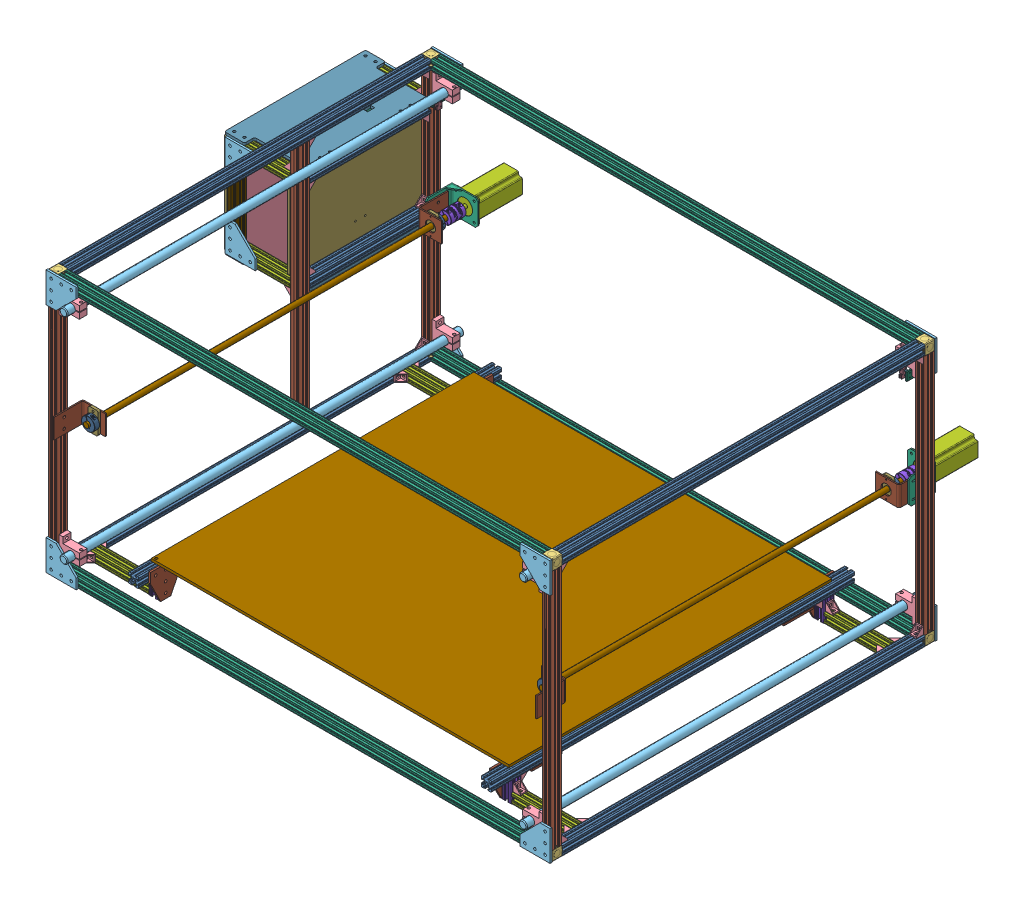
SolidWorks assembly Horizontal, configuration Default. Lengths in mm.
Overall size (1455.44 661.45 1123.18).
177 component instances, 33 part files, 21 mates.
Components (placement in the parent):
- Frame-1: Frame [Default] at origin size (1455.44 661.45 974.72)
  - Side Frame-1: Side Frame [Default] at origin size (76.73 661.45 974.72)
    - 3 ft-1: 3 ft [47065T412] at origin size (25.4 25.4 914.4)
    - 3 ft-2: 3 ft [47065T412] at (0 635 0) size (25.4 25.4 914.4)
    - 2 ft-3: 2 ft [47065T209] at (0 317.5 469.9) x (1 0 0) z (0 -1 0) size (25.4 25.4 609.6)
    - 2 ft-4: 2 ft [47065T209] at (0 317.5 -469.9) x (1 0 0) z (0 1 0) size (25.4 25.4 609.6)
    - Outside Corner-1: Outside Corner [47065T244] at (12.7 622.3 457.2) x (0 0 1) z (-1 0 0) size (28.42 28.42 28.42)
    - Outside Corner-2: Outside Corner [47065T244] at (12.7 622.3 -457.2) x (0 1 0) z (-1 0 0) size (28.42 28.42 28.42)
    - Outside Corner-3: Outside Corner [47065T244] at (12.7 12.7 457.2) x (0 -1 0) z (-1 0 0) size (28.42 28.42 28.42)
    - Outside Corner-4: Outside Corner [47065T244] at (12.7 12.7 -457.2) x (-1 0 0) z (0 -1 0) size (28.42 28.42 28.42)
    - Corner Brace-1: Corner Brace [47065T216] at (0 12.7 457.2) x (0 0 -1) z (1 0 0) size (19.81 19.81 18)
    - Corner Brace-2: Corner Brace [47065T216] at (0 12.7 -457.2) x (0 0 1) z (-1 0 0) size (19.81 19.81 18)
    - Corner Brace-3: Corner Brace [47065T216] at (0 622.3 -457.2) x (0 -1 0) z (-1 0 0) size (19.81 19.81 18)
    - Corner Brace-4: Corner Brace [47065T216] at (0 622.3 457.2) x (0 0 -1) z (-1 0 0) size (19.81 19.81 18)
    - Corner Surface-1: Corner Surface [47065T267] at (-12.7 647.7 484.9812) x (0 -1 0) z (0 0 1) size (76.2 76.2 4.76)
    - Corner Surface-3: Corner Surface [47065T267] at (-12.7 -12.7 -484.9812) size (76.2 76.2 4.76)
    - Corner Surface-4: Corner Surface [47065T267] at (-12.7 -12.7 484.9812) size (76.2 76.2 4.76)
    - Corner Surface-5: Corner Surface [47065T267] at (-12.7 647.7 -484.9812) x (0 -1 0) z (0 0 1) size (76.2 76.2 4.76)
  - 4 ft-1: 4 ft [47065T121] at (622.3 0 469.9) x (0 0 1) z (-1 0 0) size (25.4 25.4 1219.2)
  - 4 ft-2: 4 ft [47065T121] at (622.3 635 469.9) x (0 0 1) z (-1 0 0) size (25.4 25.4 1219.2)
  - 4 ft-3: 4 ft [47065T121] at (622.3 635 -469.9) x (0 0 -1) z (1 0 0) size (25.4 25.4 1219.2)
  - 4 ft-4: 4 ft [47065T121] at (622.3 0 -469.9) x (0 0 -1) z (1 0 0) size (25.4 25.4 1219.2)
  - Side Frame-2: Side Frame [Default] at (1244.6 0 0) x (-1 0 0) z (0 0 -1) size (76.73 661.45 974.72)
    - 3 ft-1: 3 ft [47065T412] at origin size (25.4 25.4 914.4)
    - 3 ft-2: 3 ft [47065T412] at (0 635 0) size (25.4 25.4 914.4)
    - 2 ft-3: 2 ft [47065T209] at (0 317.5 469.9) x (1 0 0) z (0 -1 0) size (25.4 25.4 609.6)
    - 2 ft-4: 2 ft [47065T209] at (0 317.5 -469.9) x (1 0 0) z (0 1 0) size (25.4 25.4 609.6)
    - Outside Corner-1: Outside Corner [47065T244] at (12.7 622.3 457.2) x (0 0 1) z (-1 0 0) size (28.42 28.42 28.42)
    - Outside Corner-2: Outside Corner [47065T244] at (12.7 622.3 -457.2) x (0 1 0) z (-1 0 0) size (28.42 28.42 28.42)
    - Outside Corner-3: Outside Corner [47065T244] at (12.7 12.7 457.2) x (0 -1 0) z (-1 0 0) size (28.42 28.42 28.42)
    - Outside Corner-4: Outside Corner [47065T244] at (12.7 12.7 -457.2) x (-1 0 0) z (0 -1 0) size (28.42 28.42 28.42)
    - Corner Brace-1: Corner Brace [47065T216] at (0 12.7 457.2) x (0 0 -1) z (1 0 0) size (19.81 19.81 18)
    - Corner Brace-2: Corner Brace [47065T216] at (0 12.7 -457.2) x (0 0 1) z (-1 0 0) size (19.81 19.81 18)
    - Corner Brace-3: Corner Brace [47065T216] at (0 622.3 -457.2) x (0 -1 0) z (-1 0 0) size (19.81 19.81 18)
    - Corner Brace-4: Corner Brace [47065T216] at (0 622.3 457.2) x (0 0 -1) z (-1 0 0) size (19.81 19.81 18)
    - Corner Surface-1: Corner Surface [47065T267] at (-12.7 647.7 484.9812) x (0 -1 0) z (0 0 1) size (76.2 76.2 4.76)
    - Corner Surface-3: Corner Surface [47065T267] at (-12.7 -12.7 -484.9812) size (76.2 76.2 4.76)
    - Corner Surface-4: Corner Surface [47065T267] at (-12.7 -12.7 484.9812) size (76.2 76.2 4.76)
    - Corner Surface-5: Corner Surface [47065T267] at (-12.7 647.7 -484.9812) x (0 -1 0) z (0 0 1) size (76.2 76.2 4.76)
  - 6 in-1: 6 in [47065T411] at (88.9 0 393.7) x (0 0 1) z (-1 0 0) size (25.4 25.4 152.4)
  - 2 in-3: 2 in [47065T411] at (177.8 12.7 393.7) x (1 0 0) z (0 -1 0) size (25.4 25.4 50.8)
  - 6 in-2: 6 in [47065T411] at (88.9 0 -393.7) x (0 0 -1) z (1 0 0) size (25.4 25.4 152.4)
  - 2 in-4: 2 in [47065T411] at (177.8 12.7 -393.7) x (1 0 0) z (0 1 0) size (25.4 25.4 50.8)
  - 3 ft-1: 3 ft [47065T412] at (177.8 50.8 0) size (25.4 25.4 914.4)
  - 3 ft-2: 3 ft [47065T412] at (1066.8 50.8 0) x (-1 0 0) z (0 0 -1) size (25.4 25.4 914.4)
  - 2 in-7: 2 in [47065T411] at (1066.8 12.7 393.7) x (-1 0 0) z (0 1 0) size (25.4 25.4 50.8)
  - 6 in-5: 6 in [47065T411] at (1155.7 0 393.7) x (0 0 1) z (-1 0 0) size (25.4 25.4 152.4)
  - 6 in-6: 6 in [47065T411] at (1155.7 0 -393.7) x (0 0 -1) z (1 0 0) size (25.4 25.4 152.4)
  - 2 in-8: 2 in [47065T411] at (1066.8 12.7 -393.7) x (-1 0 0) z (0 -1 0) size (25.4 25.4 50.8)
  - PVC Panel-1: PVC Panel [Default] at (622.3 66.675 0) size (901.7 6.35 812.8)
  - 34in-1: 34in [47065T412] at (622.3 50.8 -317.5) x (0 0 1) z (-1 0 0) size (25.4 25.4 863.6)
  - 34in-2: 34in [47065T412] at (622.3 50.8 317.5) x (0 0 1) z (-1 0 0) size (25.4 25.4 863.6)
  - 2 ft-1: 2 ft [47065T209] at (622.3 50.8 0) size (25.4 25.4 609.6)
  - Corner Brace-2: Corner Brace [47065T216] at (165.1 12.7 393.7) x (-1 0 0) z (0 0 -1) size (19.81 19.81 18)
  - Corner Brace-3: Corner Brace [47065T216] at (12.7 0 381) x (1 0 0) z (0 1 0) size (19.81 19.81 18)
  - Corner Brace-4: Corner Brace [47065T216] at (12.7 0 406.4) x (1 0 0) z (0 -1 0) size (19.81 19.81 18)
  - Corner Brace-5: Corner Brace [47065T216] at (177.8 38.1 381) x (0 -1 0) z (1 0 0) size (19.81 19.81 18)
  - Corner Brace-6: Corner Brace [47065T216] at (190.5 50.8 304.8) x (1 0 0) z (0 1 0) size (19.81 19.81 18)
  - Surface T-1: Surface T [47065T278] at (192.8812 63.5 355.6) x (0 0 1) z (1 0 0) size (76.2 76.2 4.76)
  - Surface T-2: Surface T [47065T278] at (165.1 35.7188 279.4) x (0 0 1) z (0 1 0) size (76.2 76.2 4.76)
  - Corner Brace-7: Corner Brace [47065T216] at (12.7 0 -406.4) x (1 0 0) z (0 1 0) size (19.81 19.81 18)
  - Corner Brace-8: Corner Brace [47065T216] at (12.7 0 -381) x (1 0 0) z (0 -1 0) size (19.81 19.81 18)
  - Corner Brace-9: Corner Brace [47065T216] at (165.1 12.7 -393.7) x (-1 0 0) z (0 0 -1) size (19.81 19.81 18)
  - Surface T-3: Surface T [47065T278] at (192.8812 63.5 -355.6) x (0 0 -1) z (-1 0 0) size (76.2 76.2 4.76)
  - Corner Brace-10: Corner Brace [47065T216] at (177.8 38.1 -381) x (0 -1 0) z (-1 0 0) size (19.81 19.81 18)
  - Surface T-4: Surface T [47065T278] at (165.1 35.7188 -279.4) x (0 0 -1) z (0 -1 0) size (76.2 76.2 4.76)
  - Corner Brace-11: Corner Brace [47065T216] at (190.5 50.8 -304.8) x (1 0 0) z (0 -1 0) size (19.81 19.81 18)
  - Corner Brace-12: Corner Brace [47065T216] at (609.6 50.8 304.8) x (-1 0 0) z (0 -1 0) size (19.81 19.81 18)
  - Surface T-5: Surface T [47065T278] at (660.4 35.7188 330.2) x (-1 0 0) z (0 -1 0) size (76.2 76.2 4.76)
  - Surface T-6: Surface T [47065T278] at (660.4 35.7188 -330.2) x (-1 0 0) z (0 1 0) size (76.2 76.2 4.76)
  - Corner Brace-13: Corner Brace [47065T216] at (609.6 50.8 -304.8) x (-1 0 0) z (0 1 0) size (19.81 19.81 18)
  - Corner Brace-14: Corner Brace [47065T216] at (1231.9 0 381) x (-1 0 0) z (0 -1 0) size (19.81 19.81 18)
  - Corner Brace-15: Corner Brace [47065T216] at (1231.9 0 406.4) x (-1 0 0) z (0 1 0) size (19.81 19.81 18)
  - Corner Brace-16: Corner Brace [47065T216] at (1231.9 0 -381) x (-1 0 0) z (0 1 0) size (19.81 19.81 18)
  - Corner Brace-17: Corner Brace [47065T216] at (1231.9 0 -406.4) x (-1 0 0) z (0 -1 0) size (19.81 19.81 18)
  - Surface T-7: Surface T [47065T278] at (1051.7188 63.5 -355.6) x (0 0 -1) z (-1 0 0) size (76.2 76.2 4.76)
  - Surface T-8: Surface T [47065T278] at (1051.7188 63.5 355.6) x (0 0 1) z (1 0 0) size (76.2 76.2 4.76)
  - Surface T-9: Surface T [47065T278] at (1079.5 35.7188 279.4) x (0 0 1) z (0 -1 0) size (76.2 76.2 4.76)
  - Surface T-10: Surface T [47065T278] at (1079.5 35.7188 -279.4) x (0 0 -1) z (0 1 0) size (76.2 76.2 4.76)
  - Corner Brace-18: Corner Brace [47065T216] at (1054.1 50.8 -304.8) x (-1 0 0) z (0 1 0) size (19.81 19.81 18)
  - Corner Brace-19: Corner Brace [47065T216] at (1054.1 50.8 304.8) x (-1 0 0) z (0 -1 0) size (19.81 19.81 18)
  - Corner Brace-20: Corner Brace [47065T216] at (1066.8 38.1 381) x (0 -1 0) z (1 0 0) size (19.81 19.81 18)
  - Corner Brace-21: Corner Brace [47065T216] at (1079.5 12.7 393.7) size (19.81 19.81 18)
  - Corner Brace-22: Corner Brace [47065T216] at (1079.5 12.7 -393.7) size (19.81 19.81 18)
  - Corner Brace-23: Corner Brace [47065T216] at (1066.8 38.1 -381) x (0 -1 0) z (-1 0 0) size (19.81 19.81 18)
  - Corner Brace-24: Corner Brace [47065T216] at (635 50.8 304.8) x (1 0 0) z (0 1 0) size (19.81 19.81 18)
  - Corner Brace-25: Corner Brace [47065T216] at (635 50.8 -304.8) x (1 0 0) z (0 -1 0) size (19.81 19.81 18)
  - Electronics Box-1: Electronics Box [Default] at (-12.7 426.5 -304.8) x (0 0 1) z (0 -1 0) size (365.12 210.31 613.21)
    - Box Bottom-1: Box Bottom [Bottom] at origin size (355.6 6.35 254)
    - Box Bottom-2: Box Bottom [Top] at (0 158.75 0) size (355.6 6.35 254)
    - Box Left-1: Box Left [Left] at (-152.4 82.55 0) x (0 0 -1) z (0 -1 0) size (254 6.35 152.4)
    - Box Left-2: Box Left [Right] at (146.05 82.55 0) x (0 0 -1) z (0 -1 0) size (254 6.35 152.4)
    - Box Front-3: Box Front [Default] at (0 69.85 127) size (355.6 190.5 6.35)
    - Box Front-4: Box Front [Back] at (0 69.85 -133.35) size (355.6 190.5 6.35)
    - Motor Drive-1: Motor Drive [Default] at (-106.05 71.23 -104.32) x (0 -1 0) z (-1 0 0) size (120 33 80)
    - Motor Drive-2: Motor Drive [Default] at (-106.05 71.23 -61.14) x (0 -1 0) z (-1 0 0) size (120 33 80)
    - Motor Drive-3: Motor Drive [Default] at (-106.05 71.23 25.22) x (0 -1 0) z (-1 0 0) size (120 33 80)
    - Motor Drive-4: Motor Drive [Default] at (-106.05 71.23 -17.96) x (0 -1 0) z (-1 0 0) size (120 33 80)
    - PSU-1: PSU [Default] at (-25 63.85 -12.7) x (0 0 -1) z (0 -1 0) size (215 50 115)
    - pi-1: pi [Default] at (80.934 6.35 15.1253) x (-1 0 0) z (0 0 -1) size (93.98 91.95 116.84)
    - Box Side Frame-1: Box Side Frame [Default] at (-165.1 146.05 0) x (-1 0 0) z (0 0 -1) size (30.16 160.56 290)
      - 8 in-1: 8 in [47065T411] at origin size (25.4 25.4 203.2)
      - 6 in-1: 6 in [47065T411] at (0 -69.85 114.3) x (1 0 0) z (0 -1 0) size (25.4 25.4 152.4)
      - 6 in-2: 6 in [47065T411] at (0 -69.85 -114.3) x (1 0 0) z (0 1 0) size (25.4 25.4 152.4)
      - Corner Surface-1: Corner Surface [47065T267] at (15.0812 12.7 127) x (0 -1 0) z (1 0 0) size (76.2 76.2 4.76)
      - Corner Surface-2: Corner Surface [47065T267] at (15.0812 12.7 -127) x (0 0 1) z (1 0 0) size (76.2 76.2 4.76)
      - Corner Brace-1: Corner Brace [47065T216] at (0 -146.05 127) x (0 0 1) z (-1 0 0) size (19.81 19.81 18)
      - Corner Brace-2: Corner Brace [47065T216] at (0 -146.05 -127) x (0 0 -1) z (1 0 0) size (19.81 19.81 18)
    - Box Side Frame-2: Box Side Frame [Default] at (165.1 146.05 0) size (30.16 160.56 290)
      - 8 in-1: 8 in [47065T411] at origin size (25.4 25.4 203.2)
      - 6 in-1: 6 in [47065T411] at (0 -69.85 114.3) x (1 0 0) z (0 -1 0) size (25.4 25.4 152.4)
      - 6 in-2: 6 in [47065T411] at (0 -69.85 -114.3) x (1 0 0) z (0 1 0) size (25.4 25.4 152.4)
      - Corner Surface-1: Corner Surface [47065T267] at (15.0812 12.7 127) x (0 -1 0) z (1 0 0) size (76.2 76.2 4.76)
      - Corner Surface-2: Corner Surface [47065T267] at (15.0812 12.7 -127) x (0 0 1) z (1 0 0) size (76.2 76.2 4.76)
      - Corner Brace-1: Corner Brace [47065T216] at (0 -146.05 127) x (0 0 1) z (-1 0 0) size (19.81 19.81 18)
      - Corner Brace-2: Corner Brace [47065T216] at (0 -146.05 -127) x (0 0 -1) z (1 0 0) size (19.81 19.81 18)
    - 2 ft-2: 2 ft [47065T209] at (165.1 -12.7 109) size (25.4 25.4 609.6)
    - 1 ft-3: 1 ft [47065T411] at (0 -12.7 114.3) x (0 0 1) z (-1 0 0) size (25.4 25.4 304.8)
    - Corner Brace-9: Corner Brace [47065T216] at (-152.4 -12.7 101.6) x (0 0 -1) z (0 -1 0) size (19.81 19.81 18)
    - Corner Brace-10: Corner Brace [47065T216] at (152.4 -12.7 101.6) x (0 0 -1) z (0 1 0) size (19.81 19.81 18)
    - 1 ft-4: 1 ft [47065T411] at (0 -12.7 -114.3) x (0 0 -1) z (1 0 0) size (25.4 25.4 304.8)
    - Corner Brace-13: Corner Brace [47065T216] at (-152.4 -12.7 -101.6) x (0 0 1) z (0 1 0) size (19.81 19.81 18)
    - Corner Brace-14: Corner Brace [47065T216] at (152.4 -12.7 -101.6) x (-1 0 0) z (0 1 0) size (19.81 19.81 18)
    - Corner Brace-15: Corner Brace [47065T216] at (152.4 -12.7 -195.8) x (0 0 1) z (0 -1 0) size (19.81 19.81 18)
    - Corner Brace-16: Corner Brace [47065T216] at (152.4 -12.7 413.8) x (-1 0 0) z (0 -1 0) size (19.81 19.81 18)
    - Switch-1: Switch [7343K291] at (25.4 158.75 -76.2) x (0 0 -1) z (1 0 0) size (31.31 51.82 16)
    - Switch-2: Switch [7343K291] at (63.5 158.75 -76.2) x (0 0 -1) z (1 0 0) size (31.31 51.82 16)
    - Switch-3: Switch [7343K291] at (101.6 158.75 -76.2) x (0 0 -1) z (1 0 0) size (31.31 51.82 16)
    - Switch Holder-1: Switch Holder [Default] at (63.5 156.083 -76.2) size (152.4 5.33 63.5)
- Horizontal Rail-1: Horizontal Rail [Default] at (12.7 79.125 469.9) x (0 -1 0) z (0 0 1) size (60 51 1000)
  - Shaft Clamp 20mm-1: Shaft Clamp 20mm [Default] at (0 0 -939.8) size (60 51 20)
  - Shaft 1000mm-1: Shaft 1000mm [6459K62] at (30 31 -469.9) x (-0.976033 -0.217622 0) z (0 0 1) size (20 20 1000)
  - Shaft Clamp 20mm-11: Shaft Clamp 20mm [Default] at origin size (60 51 20)
- Horizontal Motor-1: Horizontal Motor [Default] at (48.2 319.125 -510.1768) x (0 -1 0) z (0 0 1) size (65 68 1118.48)
  - Motor Mount-1: Motor Mount [Default] at origin size (65 68 68)
  - Nema 23 Stepper Motor-1: Nema 23 Stepper Motor [Default] at (28.5 -28.5 0) x (0 0 -1) z (1 0 0) size (137 57 57)
  - Shaft Coupler-1: Shaft Coupler [2464K34] at (0 0 33.602) x (-0.85098 -0.525198 0) z (0 0 -1) size (30 30.01 38)
  - Lead Screw 3ft-2: Lead Screw 3ft [Default] at (0 0 500.404) x (0 0 1) z (0.598663 0.801001 0) size (914.4 12.7 12.7)
  - Collar-1: Collar [6698K13] at (0 0 74.1796) x (0.295803 -0.955249 0) z (0 0 1) size (33.3 33.27 13.41)
  - Collar-2: Collar [6698K13] at (0 0 946.174) x (0.943106 0.332491 0) z (0 0 1) size (33.3 33.27 13.41)
  - L Bracket-1: L Bracket [Without Motor] at (25 -35.5 930.4768) x (0 0 1) z (-1 0 0) size (75 59.99 50)
  - L Bracket-2: L Bracket [With Motor] at (-25 -32.5 89.8768) x (0 0 -1) z (1 0 0) size (75 59.99 50)
  - Acrylic Bearing Mount-1: Acrylic Bearing Mount [Default] at (0 0 936.649) size (55.88 25.4 6.35)
  - Acrylic Bearing Mount-2: Acrylic Bearing Mount [Default] at (0 0 83.7046) size (55.88 25.4 6.35)
- Horizontal Rail-3: Horizontal Rail [Default] at (12.7 619.125 469.9) x (0 -1 0) z (0 0 1) size (60 51 1000)
  - Shaft Clamp 20mm-1: Shaft Clamp 20mm [Default] at (0 0 -939.8) size (60 51 20)
  - Shaft 1000mm-1: Shaft 1000mm [6459K62] at (30 31 -469.9) x (-0.976033 -0.217622 0) z (0 0 1) size (20 20 1000)
  - Shaft Clamp 20mm-11: Shaft Clamp 20mm [Default] at origin size (60 51 20)
- Limit Swtich Assembly 2-1: Limit Swtich Assembly 2 [Default] at (1221.9 571.6895 -443.7567) x (0 0 -1) z (0 1 0) size (15.52 14.29 21.84)
  - Limit Switch-2: Limit Switch [Default] at (13.2909 14.2875 -7.4832) x (0 0 1) z (0 -1 0) size (21.84 15.52 6.35)
  - Standoff-1: Standoff [90268A203] at (10.9033 11.1125 -2.7207) x (0.90245 0 -0.430795) z (0 1 0) size (4.76 5.5 7.94)
  - Standoff-2: Standoff [90268A203] at (10.9033 11.1125 -12.2457) x (0.948451 0 0.316923) z (0 1 0) size (4.76 5.5 7.94)
- Horizontal Rail-4: Horizontal Rail [Default] at (1231.9 79.125 -469.9) x (0 -1 0) z (0 0 -1) size (60 51 1000)
  - Shaft Clamp 20mm-1: Shaft Clamp 20mm [Default] at (0 0 -939.8) size (60 51 20)
  - Shaft 1000mm-1: Shaft 1000mm [6459K62] at (30 31 -469.9) x (-0.976033 -0.217622 0) z (0 0 1) size (20 20 1000)
  - Shaft Clamp 20mm-11: Shaft Clamp 20mm [Default] at origin size (60 51 20)
- Horizontal Motor-2: Horizontal Motor [Default] at (1196.4 319.125 -510.1768) x (0 1 0) z (0 0 1) size (65 68 1118.48)
  - Motor Mount-1: Motor Mount [Default] at origin size (65 68 68)
  - Nema 23 Stepper Motor-1: Nema 23 Stepper Motor [Default] at (28.5 -28.5 0) x (0 0 -1) z (1 0 0) size (137 57 57)
  - Shaft Coupler-1: Shaft Coupler [2464K34] at (0 0 33.602) x (-0.85098 -0.525198 0) z (0 0 -1) size (30 30.01 38)
  - Lead Screw 3ft-2: Lead Screw 3ft [Default] at (0 0 500.404) x (0 0 1) z (0.598663 0.801001 0) size (914.4 12.7 12.7)
  - Collar-1: Collar [6698K13] at (0 0 74.1796) x (0.295803 -0.955249 0) z (0 0 1) size (33.3 33.27 13.41)
  - Collar-2: Collar [6698K13] at (0 0 946.174) x (0.943106 0.332491 0) z (0 0 1) size (33.3 33.27 13.41)
  - L Bracket-1: L Bracket [Without Motor] at (25 -35.5 930.4768) x (0 0 1) z (-1 0 0) size (75 59.99 50)
  - L Bracket-2: L Bracket [With Motor] at (-25 -32.5 89.8768) x (0 0 -1) z (1 0 0) size (75 59.99 50)
  - Acrylic Bearing Mount-1: Acrylic Bearing Mount [Default] at (0 0 936.649) size (55.88 25.4 6.35)
  - Acrylic Bearing Mount-2: Acrylic Bearing Mount [Default] at (0 0 83.7046) size (55.88 25.4 6.35)
- Horizontal Rail-5: Horizontal Rail [Default] at (1231.9 619.125 -469.9) x (0 -1 0) z (0 0 -1) size (60 51 1000)
  - Shaft Clamp 20mm-1: Shaft Clamp 20mm [Default] at (0 0 -939.8) size (60 51 20)
  - Shaft 1000mm-1: Shaft 1000mm [6459K62] at (30 31 -469.9) x (-0.976033 -0.217622 0) z (0 0 1) size (20 20 1000)
  - Shaft Clamp 20mm-11: Shaft Clamp 20mm [Default] at origin size (60 51 20)
- Limit Swtich Assembly 1-2: Limit Swtich Assembly 1 [Default] at (21.8635 571.2553 -445.7389) x (0 0 -1) z (0 1 0) size (15.52 14.29 21.84)
  - Limit Switch-2: Limit Switch [Default] at (11.3087 -15.124 -7.049) x (0 0 1) z (0 -1 0) size (21.84 15.52 6.35)
  - Standoff-1: Standoff [90268A203] at (8.9211 -4.0115 -2.2865) x (0.645868 0 0.763449) z (0 1 0) size (4.76 5.5 7.94)
  - Standoff-2: Standoff [90268A203] at (8.9211 -4.0115 -11.8115) x (0.926416 0 0.3765) z (0 1 0) size (4.76 5.5 7.94)
- Al sheet 4-1-1: Al sheet 4-1 [Default] at (1221.9 574.125 -446.88) x (0 0 -1) z (0 1 0) size (33.02 3.17 20.32)
- Al sheet 4-1-2: Al sheet 4-1 [Default] at (25.875 574.125 -446.88) x (0 0 -1) z (0 1 0) size (33.02 3.17 20.32)
Mates (geometry in assembly coordinates):
- Coincident1: coincident anti-aligned: plane of Frame-1/Side Frame-1/2 ft-3 through (12.7 12.7 460.3496) normal (1 0 0); plane of Horizontal Rail-3/Shaft Clamp 20mm-11 through (12.7 619.125 479.9) normal (-1 0 0)
- Coincident3: coincident aligned: plane of Frame-1/Side Frame-1/2 ft-3 through (0 317.5 469.9) normal (0 0 1); plane of Horizontal Rail-3/Shaft Clamp 20mm-11 through (12.7 619.125 469.9) normal (0 0 1)
- Distance5: distance = 3.175 mm anti-aligned: plane of Frame-1/4 ft-2 through (12.7 622.3 476.2331) normal (0 -1 0); plane of Horizontal Rail-3/Shaft Clamp 20mm-11 through (12.7 619.125 479.9) normal (0 1 0)
- Coincident5: coincident anti-aligned: plane of Frame-1/Side Frame-1/2 ft-3 through (12.7 12.7 460.3496) normal (1 0 0); plane of Horizontal Rail-1/Shaft Clamp 20mm-11 through (12.7 79.125 479.9) normal (-1 0 0)
- Coincident6: coincident aligned: plane of Frame-1/Side Frame-1/2 ft-3 through (0 317.5 469.9) normal (0 0 1); plane of Horizontal Rail-1/Shaft Clamp 20mm-11 through (12.7 79.125 469.9) normal (0 0 1)
- Coincident7: coincident anti-aligned: plane of Frame-1/Side Frame-1/2 ft-3 through (12.7 12.7 460.3496) normal (1 0 0); plane of Horizontal Motor-1/L Bracket-1 through (12.7 344.125 426.142) normal (-1 0 0)
- Distance1: distance = 12.7 mm aligned: plane of Horizontal Motor-1/L Bracket-1 through (15.6972 344.125 495.3) normal (0 0 1); plane of Frame-1/Side Frame-1/2 ft-3 through (9.5504 12.7 482.6) normal (0 0 1)
- Distance2: distance = 520 mm: cylinder of Horizontal Rail-3/Shaft 1000mm-1 through (43.7 589.125 500) axis (0 0 -1) radius 10; cylinder of Horizontal Rail-1/Shaft 1000mm-1 through (43.7 49.125 500) axis (0 0 -1) radius 10
- Distance3: distance = 215 mm anti-aligned: plane of Horizontal Rail-3/Shaft Clamp 20mm-11 through (12.7 559.125 479.9) normal (0 -1 0); plane of Horizontal Motor-1/L Bracket-1 through (18.8722 344.125 426.4722) normal (0 1 0)
- Concentric2: concentric anti-aligned: circle of Limit Swtich Assembly 2-1/Standoff-2; cylinder of Al sheet 4-1-1 through (1221.9 559.4438 -454.66) axis (-1 0 0) radius 1.1303
- Concentric3: concentric anti-aligned: circle of Limit Swtich Assembly 2-1/Standoff-1; cylinder of Al sheet 4-1-1 through (1221.9 568.9688 -454.66) axis (-1 0 0) radius 1.1303
- Coincident10: coincident anti-aligned: plane of Limit Swtich Assembly 2-1/Standoff-2 through (1218.725 554.7773 -453.7086) normal (1 0 0); plane of Al sheet 4-1-1 through (1218.725 574.125 -446.88) normal (-1 0 0)
- Concentric5: concentric aligned: circle of Limit Swtich Assembly 1-2/Standoff-2; cylinder of Al sheet 4-1-2 through (25.875 559.4438 -454.66) axis (-1 0 0) radius 1.1303
- Concentric6: concentric aligned: circle of Limit Swtich Assembly 1-2/Standoff-1; circle of Al sheet 4-1-2
- Coincident13: coincident anti-aligned: plane of Limit Swtich Assembly 1-2/Standoff-1 through (25.875 564.487 -456.2708) normal (-1 0 0); plane of Al sheet 4-1-2 through (25.875 574.125 -446.88) normal (1 0 0)
- Coincident14: coincident anti-aligned: plane of Horizontal Rail-5/Shaft Clamp 20mm-11 through (1221.9 574.125 -479.9) normal (-1 0 0); plane of Al sheet 4-1-1 through (1221.9 574.125 -446.88) normal (1 0 0)
- Concentric7: concentric anti-aligned: cylinder of Horizontal Rail-5/Shaft Clamp 20mm-11 through (1247.9 566.625 -469.9) axis (-1 0 0) radius 3.3; cylinder of Al sheet 4-1-1 through (1218.725 566.625 -469.9) axis (1 0 0) radius 3.3
- Coincident15: coincident anti-aligned: plane of Horizontal Rail-5/Shaft Clamp 20mm-11 through (1221.9 574.125 -479.9) normal (0 -1 0); plane of Al sheet 4-1-1 through (1218.725 574.125 -446.88) normal (0 1 0)
- Coincident17: coincident anti-aligned: plane of Horizontal Rail-3/Shaft Clamp 20mm-1 through (22.7 574.125 -459.9) normal (1 0 0); plane of Al sheet 4-1-2 through (22.7 574.125 -446.88) normal (-1 0 0)
- Concentric8: concentric aligned: cylinder of Horizontal Rail-3/Shaft Clamp 20mm-1 through (-3.3 566.625 -469.9) axis (1 0 0) radius 3.3; cylinder of Al sheet 4-1-2 through (22.7 566.625 -469.9) axis (1 0 0) radius 3.3
- Coincident18: coincident anti-aligned: plane of Horizontal Rail-3/Shaft Clamp 20mm-1 through (22.7 574.125 -459.9) normal (0 -1 0); plane of Al sheet 4-1-2 through (22.7 574.125 -446.88) normal (0 1 0)
